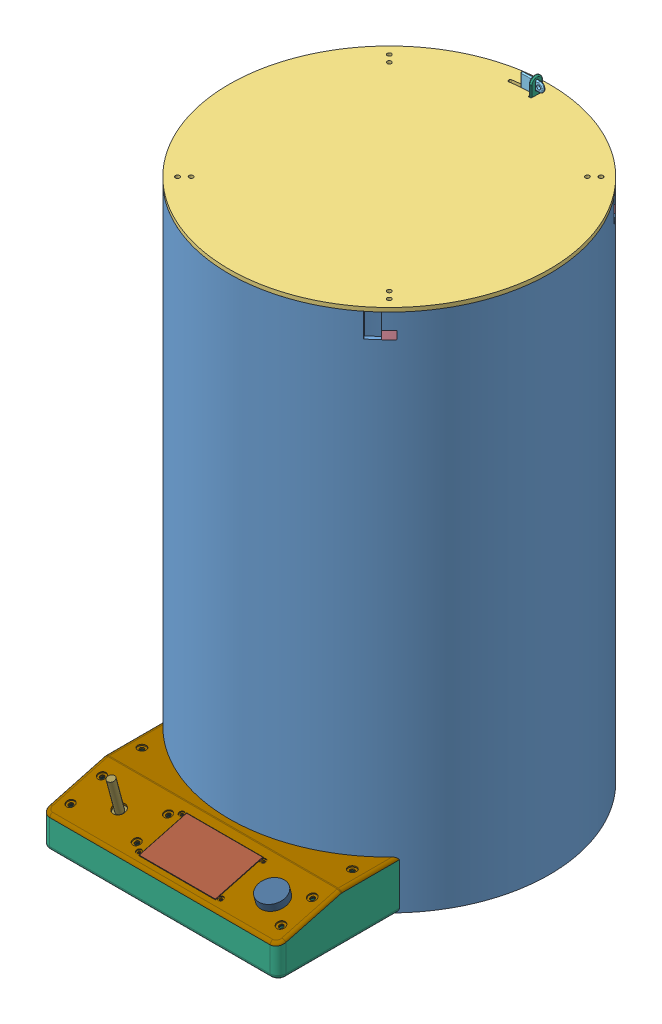
SolidWorks assembly 装配体, configuration 默认. Lengths in mm.
Overall size (565.69 675.37 570.66).
79 component instances, 42 part files, 24 mates.
Components (placement in the parent):
- 侧壁-1: 侧壁 [默认] at origin size (400 650 400)
- 出球口平台-2: 出球口平台 [默认] at (0 346.4 0) x (1 0 0) z (0 0 -1) size (112.05 40.22 152.95)
- 顶盖-1: 顶盖 [默认] at (0 650 0) x (0.707107 0 -0.707107) z (0.707107 0 0.707107) size (400 195.14 400)
  - 顶盖-1: 顶盖 [默认] at origin size (400 5 400)
  - 顶盖L锁-5: 顶盖L锁 [默认] at (0 -30 0) size (13.96 30 35)
  - 顶盖L锁-6: 顶盖L锁 [默认] at (0 -30 0) x (0 0 -1) z (1 0 0) size (13.96 30 35)
  - 顶盖L锁-7: 顶盖L锁 [默认] at (0 -30 0) x (-1 0 0) z (0 0 -1) size (13.96 30 35)
  - 顶盖L锁-8: 顶盖L锁 [默认] at (0 -30 0) x (0 0 1) z (-1 0 0) size (13.96 30 35)
  - 滑轨-1: 滑轨 [默认] at (0 -15 0) x (0.707107 0 0.707107) z (-0.707107 0 0.707107) size (370 15 15)
  - 滑块-1: 滑块 [默认] at (108.0892 -15 108.0892) x (-0.707107 0 -0.707107) z (-0.707107 0 0.707107) size (62.3 13 34)
  - 滑块止动块-1: 滑块止动块 [默认] at (154.4664 -15 154.4664) x (0.707107 0 0.707107) z (-0.707107 0 0.707107) size (9 15 15)
  - 滑块止动块-2: 滑块止动块 [默认] at (-154.4664 -15 -154.4664) x (-0.707107 0 -0.707107) z (0.707107 0 -0.707107) size (9 15 15)
  - 皮带主动轮-1: 皮带主动轮 [默认] at (-68.0499 0 -174.1733) x (-0.707107 0 0.707107) z (0.707107 0 0.707107) size (49.4 30.75 25.6)
    - 皮带主动轮架-1: 皮带主动轮架 [默认] at origin size (25.5 14 25.6)
    - N20减速电机-1: N20减速电机 [默认] at (16.7906 14 0) size (35.3 11.4 25.6)
    - 皮带轮-1: 皮带轮 [默认] at (53.4406 19 0) x (0 -0.381849 0.924225) z (0 -0.924225 -0.381849) size (18 22.4 18)
  - 皮带从动轮-1: 皮带从动轮 [默认] at (151.9382 0 105.6227) x (0.707107 0 -0.707107) z (-0.707107 0 -0.707107) size (29.5 31.64 25.28)
    - 皮带从动轮架-1: 皮带从动轮架 [默认] at origin size (29.5 23.4 12)
    - 皮带轮-1: 皮带轮 [默认] at (-11.15 19 0) x (0 0.620152 -0.784482) z (0 -0.784482 -0.620152) size (18 22.4 18)
  - 皮带1-3^顶盖-1: 皮带1-3^顶盖 [默认] at (-100.8883 -19 -141.3349) x (0.707107 0 0.707107) z (-0.707107 0 0.707107) size (373.4 20 10) (virtual)
  - 吊轮-1: 吊轮 [默认] at (108.0892 -28 108.0892) x (-0.707107 0 -0.707107) z (-0.707107 0 0.707107) size (64.3 135.96 77.73)
    - 吊轮架-1: 吊轮架 [默认] at origin size (62.3 80.1 77.6)
    - 皮带扣-1: 皮带扣 [默认] at (0 -8.27 -28.6) size (22.72 7.07 22.66)
    - N20减速电机-1: N20减速电机 [默认] at (0 19 25.05) x (0 0 -1) z (1 0 0) size (35.3 11.4 25.6)
    - 线轮-1: 线轮 [默认] at (0 24 0) x (0.313692 -0.949525 0) z (0 0 1) size (38 38 10)
    - 导电滑环-紧凑-1: 导电滑环-紧凑 [默认] at (0 24 -2.5) x (0 0 -1) z (-0.020009 -0.9998 0) size (13.5 6.5 6.5)
    - 电磁铁架-1: 电磁铁架 [默认] at (2.1 55.1442 0) x (0 0 -1) z (-1 0 0) size (41.4 73.75 41.4)
      - 电磁铁架-1: 电磁铁架 [默认] at origin size (21 20 6.65)
      - 导线扣-1: 导线扣 [默认] at (0 0 2.5) size (21 10 1.5)
      - 电磁铁-1: 电磁铁 [默认] at (0 -68.75 2.1) x (-0.999364 0 0.035666) z (-0.035666 0 -0.999364) size (40 55 40)
    - 红外接近开关-1: 红外接近开关 [默认] at (-27.65 50.5 0) x (0 -1 0) z (0 0 1) size (31.2 18 14)
  - 灯条-1: 灯条 [默认] at (-34.2947 0 34.2947) x (0.707107 0 -0.707107) z (0 -1 0) size (37 328.51 17)
    - 灯条-1: 灯条 [默认] at origin size (20 303 15.5)
    - 灯条固定架1-1: 灯条固定架1 [默认] at (0 -151.5 8.5) x (-1 0 0) z (0 1 0) size (37 17 19.1)
    - 灯条固定架2-1: 灯条固定架2 [默认] at (0 151.5 8.5) x (1 0 0) z (0 -1 0) size (37 17 19.41)
  - 铁球-1: 铁球 [默认] at (108.0892 -155.1382 108.0892) x (0.707107 0 -0.707107) z (0.707107 0 0.707107) size (70 70 70) (hidden)
  - 红外接近开关-1: 红外接近开关 [默认] at (96.8104 -20.4 139.2368) x (0 1 0) z (-0.707107 0 0.707107) size (31.2 18 14)
  - 红外接近开关-2: 红外接近开关 [默认] at (-136.8155 -20.4 -94.3891) x (0 1 0) z (0.707107 0 -0.707107) size (31.2 18 14)
- 底座-2: 底座 [默认] at (0 0 240) size (389 346.4 482.37)
  - 底盘-1: 底盘 [默认] at origin size (389 93.4 481.16)
    - 底盘-1: 底盘 [默认] at origin size (389 87.9 481.16)
    - 底盘电机-1: 底盘电机 [默认] at (-7.95 18.6 -224.2) x (-1 0 0) z (0 0 -1) size (77.9 89.9 37.9)
    - 开关电源-1: 开关电源 [默认] at (0 3 -319.3) x (0 0 1) z (-1 0 0) size (98 38 200)
  - 操纵台-1: 操纵台 [默认] at (12.35 47 6.5226) x (-1 0 0) z (0 0 -1) size (296.13 98.31 152.91)
    - 操纵台顶盖-1: 操纵台顶盖 [默认] at origin size (296.13 47.95 151.7)
    - 按钮-1: 按钮 [默认] at (-90.3 2.799 -0.75) x (1 0 0) z (0 0.258819 0.965926) size (32.6 32 32.6)
    - 显示屏2-1: 显示屏2 [默认] at (0 -2.8012 0.7506) x (-1 0 0) z (0 -0.258819 -0.965926) size (108 14.6 61.7)
    - 摇杆-1: 摇杆 [默认] at (102.5 -1.1591 0.3106) x (-1 0 0) z (0 -0.258819 -0.965926) size (95 78.2 88)
    - M3弹簧垫圈-1: M3弹簧垫圈 [默认] at (51 6.3448 26.77) x (1 0 0) z (0 0.258819 0.965926) size (5 0.8 5)
    - M3弹簧垫圈-5: M3弹簧垫圈 [默认] at (-51 -7.8903 -26.3559) x (1 0 0) z (0 0.258819 0.965926) size (5 0.8 5)
    - M3弹簧垫圈-6: M3弹簧垫圈 [默认] at (-51 6.3448 26.77) x (1 0 0) z (0 0.258819 0.965926) size (5 0.8 5)
    - M3弹簧垫圈-7: M3弹簧垫圈 [默认] at (51 -7.8903 -26.3559) x (1 0 0) z (0 0.258819 0.965926) size (5 0.8 5)
    - 垫圈M3x5x0.5-1: 垫圈M3x5x0.5 [默认] at (51 5.8618 26.8994) x (0.98005 0.051441 0.191979) z (-0.198752 0.253656 0.946656) size (5 0.5 5)
    - 垫圈M3x5x0.5-2: 垫圈M3x5x0.5 [默认] at (-51 -8.3732 -26.2265) x (0.98005 0.051441 0.191979) z (-0.198752 0.253656 0.946656) size (5 0.5 5)
    - 垫圈M3x5x0.5-3: 垫圈M3x5x0.5 [默认] at (-51 5.8618 26.8994) x (0.98005 0.051441 0.191979) z (-0.198752 0.253656 0.946656) size (5 0.5 5)
    - 垫圈M3x5x0.5-4: 垫圈M3x5x0.5 [默认] at (51 -8.3732 -26.2265) x (0.98005 0.051441 0.191979) z (-0.198752 0.253656 0.946656) size (5 0.5 5)
  - M5弹簧垫圈-1: M5弹簧垫圈 [默认] at (-131.4 49.8651 -13.8293) x (0.894459 -0.115731 0.431914) z (-0.44715 -0.231503 0.863981) size (8 1.3 8)
  - M5弹簧垫圈-8: M5弹簧垫圈 [默认] at (-48.8 39.3829 25.2907) x (0.894459 -0.115731 0.431914) z (-0.44715 -0.231503 0.863981) size (8 1.3 8)
  - M5弹簧垫圈-9: M5弹簧垫圈 [默认] at (-48.8 49.8651 -13.8293) x (0.894459 -0.115731 0.431914) z (-0.44715 -0.231503 0.863981) size (8 1.3 8)
  - M5弹簧垫圈-10: M5弹簧垫圈 [默认] at (-131.4 39.3829 25.2907) x (0.894459 -0.115731 0.431914) z (-0.44715 -0.231503 0.863981) size (8 1.3 8)
  - M5弹簧垫圈-11: M5弹簧垫圈 [默认] at (131.4 40.542 25.6013) x (0.894459 -0.115731 0.431914) z (-0.44715 -0.231503 0.863981) size (8 1.3 8)
  - M5弹簧垫圈-12: M5弹簧垫圈 [默认] at (131.4 51.0242 -13.5187) x (0.894459 -0.115731 0.431914) z (-0.44715 -0.231503 0.863981) size (8 1.3 8)
  - M5弹簧垫圈-13: M5弹簧垫圈 [默认] at (-131.4 56.1433 -62.4525) size (8 1.3 8)
  - M5弹簧垫圈-14: M5弹簧垫圈 [默认] at (131.4 56.1433 -62.4525) size (8 1.3 8)
  - 转盘-1: 转盘 [默认] at (0 88.4 -240) size (380 258 380)
    - 转盘-1: 转盘 [默认] at origin size (380 3 380)
    - 塔-1: 塔 [默认] at (0 3 0) size (100 255 100)
    - 挡板-1: 挡板 [默认] at (-130 20.5 1) x (-1 0 0) z (0 0 -1) size (120 36.5 18)
    - 挡板-2: 挡板 [默认] at (64.134 20.5 -113.0833) x (0.5 0 -0.866025) z (0.866025 0 0.5) size (120 36.5 18)
    - 挡板-3: 挡板 [默认] at (65.866 20.5 112.0833) x (0.5 0 0.866025) z (-0.866025 0 0.5) size (120 36.5 18)
- 铁球-1: 铁球 [默认] at (159.7836 126.4 8.3189) x (0.914982 -0.39772 -0.068015) z (0.387475 0.81906 0.423089) size (70 70 70)
- 大铁盒-1: 大铁盒 [默认] at (-30.0581 91.4 -106.8473) size (94 90 94)
- 大铁盒-2: 大铁盒 [默认] at (-139.7008 408.1058 1.8998) size (94 90 94)
- 小铁盒-1: 小铁盒 [默认] at (-5.8943 91.4 106.8666) size (75 65 75)
- RGB灯带 圆形-1: RGB灯带 圆形 [默认] at (0 121.0738 0) size (390 20 390)
- RGB灯带 圆形-2: RGB灯带 圆形 [默认] at (0 560.7459 0) size (390 20 390)
- 顶盖-侧壁连接器-1: 顶盖-侧壁连接器 [默认] at (0 642 0) x (-1 0 0) z (0 0 -1) size (52.82 67.64 24)
  - 侧壁密码锁-2: 侧壁密码锁 [默认] at (0 -30 0) x (0.999048 0 -0.043619) z (0.043619 0 0.999048) size (29.4 63.61 16.3)
  - 顶盖密码锁-1: 顶盖密码锁 [默认] at origin size (35.76 33.42 17.63)
Mates (geometry in assembly coordinates):
- 重合19: coincident anti-aligned: plane of 侧壁-1 through (0 650 0) normal (0 1 0); plane of 顶盖-1/顶盖-1 through (0 650 0) normal (0 -1 0)
- 同心29: concentric aligned: cylinder of 侧壁-1 through (0 650 0) axis (0 -1 0) radius 195; cylinder of 顶盖-1/顶盖-1 through (0 655 0) axis (0 -1 0) radius 200
- 重合21: coincident aligned: plane of 侧壁-1 through (0 0 0) normal (0 0 1); plane of 顶盖-1 through (0 650 0) normal (0 0 1)
- 重合26: coordinate: unknown of 侧壁-1
- 重合27: coincident aligned: plane of 侧壁-1 through (0 0 0) normal (0 0 1)
- 重合28: coincident aligned: plane of 侧壁-1 through (0 0 0) normal (0 1 0)
- 平行2: parallel aligned: plane of 底座-2 through (0 0 240) normal (0 0 1)
- 重合30: coincident aligned: plane of 侧壁-1 through (0 0 0) normal (0 -1 0); plane of 底座-2/底盘-1/底盘-1 through (0 0 240) normal (0 -1 0)
- 同心31: concentric aligned: cylinder of 侧壁-1 through (0 650 0) axis (0 -1 0) radius 200; cylinder of 底座-2/底盘-1/底盘-1 through (0 3 0) axis (0 -1 0) radius 194.5
- 重合40: coincident anti-aligned: plane of 出球口平台-2 through (0 346.4 0) normal (0 0 -1)
- 重合41: coincident anti-aligned: plane of 出球口平台-2 through (0 346.4 0) normal (0 -1 0)
- 重合42: coincident aligned: plane of 出球口平台-2 through (0 346.4 0) normal (1 0 0)
- 相切1: tangent anti-aligned: plane of 底座-2/转盘-1/转盘-1 through (0 91.4 0) normal (0 1 0); sphere of 铁球-1
- 相切2: tangent aligned: cylinder of 侧壁-1 through (0 650 0) axis (0 -1 0) radius 195; sphere of 铁球-1
- 重合43: coincident anti-aligned: plane of 底座-2/转盘-1/转盘-1 through (0 91.4 0) normal (0 1 0); plane of 大铁盒-1 through (-30.0581 91.4 -106.8473) normal (0 -1 0)
- 重合45: coincident anti-aligned: plane of 底座-2/转盘-1/转盘-1 through (0 91.4 0) normal (0 1 0); plane of 小铁盒-1 through (-5.8943 91.4 106.8666) normal (0 -1 0)
- 重合46: coincident anti-aligned: plane of 顶盖-1/吊轮-1/电磁铁架-1/电磁铁-1 through (152.8613 498.1058 0) normal (0 -1 0); plane of 大铁盒-2 through (-139.7008 498.1058 1.8998) normal (0 1 0)
- 重合47: coincident aligned: plane of RGB灯带 圆形-1 through (0 121.0738 0) normal (0 0 1)
- 重合48: coincident aligned: plane of RGB灯带 圆形-1 through (0 121.0738 0) normal (1 0 0)
- 重合49: coincident aligned: plane of RGB灯带 圆形-2 through (0 560.7459 0) normal (0 0 1)
- 重合50: coincident aligned: plane of RGB灯带 圆形-2 through (0 560.7459 0) normal (1 0 0)
- 同心32: concentric aligned: cylinder of 侧壁-1 through (0 650 0) axis (0 -1 0) radius 195; cylinder of 顶盖-侧壁连接器-1/侧壁密码锁-2 through (0 647 0) axis (0 -1 0) radius 195
- 重合51: coincident anti-aligned: plane of 顶盖-1/顶盖-1 through (0 650 0) normal (0 -1 0); plane of 顶盖-侧壁连接器-1/侧壁密码锁-2 through (0 650 0) normal (0 1 0)
- 重合52: coincident anti-aligned: plane of 顶盖-侧壁连接器-1 through (0 642 0) normal (-1 0 0)
